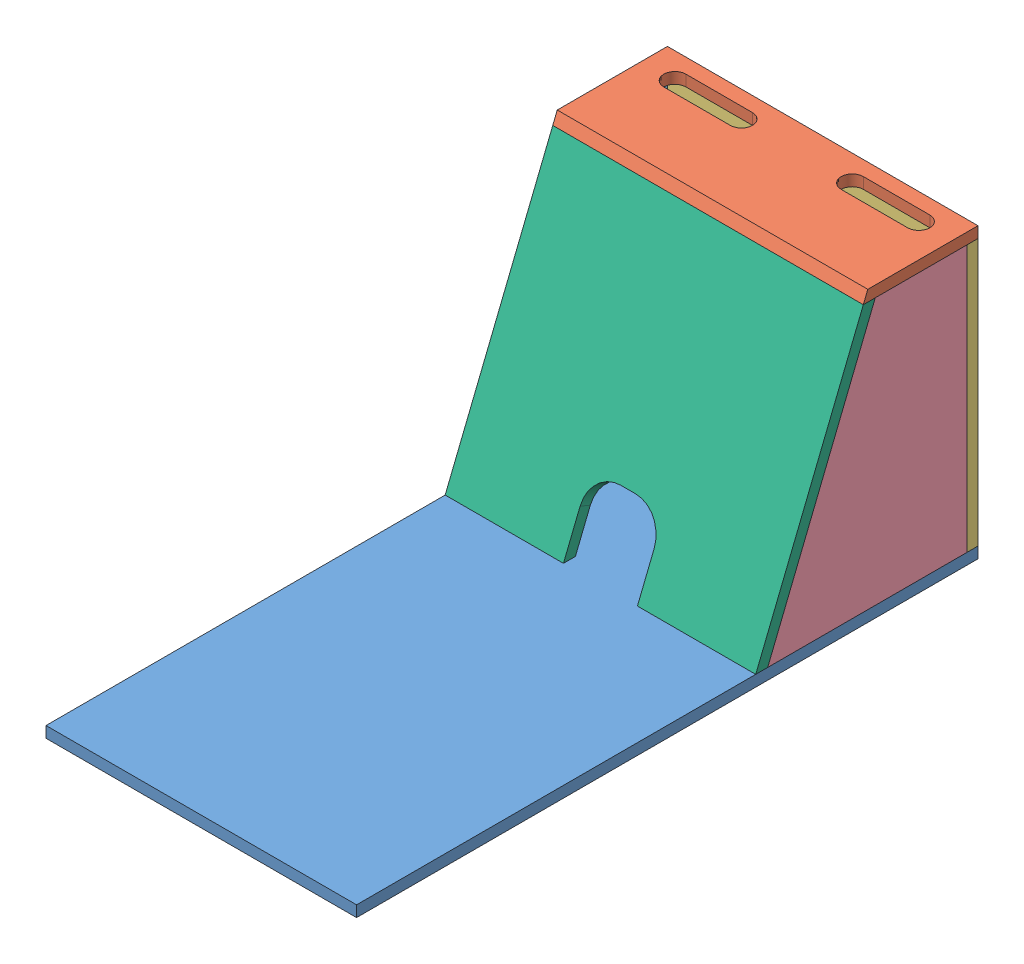
SolidWorks assembly Center Tub, configuration Default. Lengths in mm.
Overall size (533.15 495.3 1066.8).
6 component instances, 6 part files, 17 mates.
Components (placement in the parent):
- Center Tub Floor-1: Center Tub Floor [Default] at (0 2664.46 0) x (-1 0 0) z (0 -1 0) size (533.15 1066.8 19.05)
- Center Tub Keystone-1: Center Tub Keystone [Default] at origin size (533.15 19.05 196.86)
- Center Tub Aft Bulkhead-1: Center Tub Aft Bulkhead [Default] at (0 0 -7002.78) x (-1 0 0) z (0 0 -1) size (533.15 457.2 19.05)
- Center Tub Left Wall-1: Center Tub Left Wall [Default] at (266.573 0 0) x (0 1 0) z (-1 0 0) size (457.2 341.99 19.05)
- Center Tub Right Wall-2: Center Tub Right Wall [Default] at (-266.573 0 0) x (0 1 0) z (-1 0 0) size (457.2 341.99 19.05)
- Center Tub FWD Bulkhead-1: Center Tub FWD Bulkhead [Default] at (-266.573 -1930.2936 -4777.6442) x (0 -0.927184 0.374607) z (0 0.374607 0.927184) size (500.8 533.15 19.05)
Mates (geometry in assembly coordinates):
- InPlace1: in place: plane of ? through (266.7 3017.195 -6812.7359) normal (-1 0 0); plane of ? through (266.7 0 0) normal (-1 0 0); moOrthogonalPlaneRef_w of ? through (266.7 3017.195 -6812.7359) normal (-1 0 0); plane of ? through (266.7 0 0) normal (0 1 0); plane of ? through (266.7 3017.195 -6812.7359) normal (-1 0 0); plane of ? through (266.7 0 0) normal (0 0 1); plane of ? through (266.7 0 0) normal (-1 0 0); unknown of ?
- Coincident1: coincident aligned: plane of ?; plane of assembly
- Coincident2: coincident aligned: plane of Part5^Center Tub-1 through (266.7 0 0) normal (0 0 -1); moOrthogonalPlaneRef_w of Left Console-1/Left Console Structure-1/Inboard Left Console Wall-1 through (266.7 0 0) normal (0 0 -1)
- Coincident3: coincident anti-aligned: plane of Part5^Center Tub-1 through (266.7 0 0) normal (0 1 0); moOrthogonalPlaneRef_w of Left Console-1/Left Console Structure-1/Inboard Left Console Wall-1 through (266.7 0 0) normal (0 -1 0)
- Coincident1: coincident anti-aligned: plane of Center Tub Floor-1 through (0 2683.51 0) normal (0 1 0); plane of Center Tub Left Wall-1 through (247.523 2683.51 -6983.73) normal (0 -1 0)
- Coincident2: coincident aligned: plane of Center Tub Aft Bulkhead-1 through (266.573 2683.51 -6983.73) normal (1 0 0); plane of Center Tub Left Wall-1 through (266.573 0 0) normal (1 0 0)
- Coincident3: coincident anti-aligned: plane of Center Tub Aft Bulkhead-1 through (0 0 -6983.73) normal (0 0 1); plane of Center Tub Left Wall-1 through (247.523 3140.71 -6983.73) normal (0 0 -1)
- InPlace2: in place: plane of ? through (-247.65 2683.51 -6641.7419) normal (0 0.374607 0.927184); plane of ? through (0 -1930.2936 -4777.6442) normal (0 0.374607 0.927184); plane of ? through (-247.65 2683.51 -6641.7419) normal (0 0.374607 0.927184); plane of ? through (0 -1930.2936 -4777.6442) normal (0 0.927184 -0.374607); plane of ? through (-247.65 2683.51 -6641.7419) normal (0 0.374607 0.927184); plane of ? through (0 -1930.2936 -4777.6442) normal (1 0 0); plane of Center Tub Right Wall-2 through (-247.523 2683.51 -6641.7419) normal (0 0.374607 0.927184); unknown of Center Tub FWD Bulkhead-1
- Coincident4: coincident aligned: plane of Center Tub Right Wall-2; plane of Center Tub FWD Bulkhead-1
- Coincident5: coincident aligned: moOrthogonalPlaneRef_w of Center Tub Right Wall-2 through (-266.573 -1930.2936 -4777.6442) normal (1 0 0); plane of Center Tub FWD Bulkhead-1 through (-266.573 -1930.2936 -4777.6442) normal (1 0 0)
- Coincident6: coincident anti-aligned: moOrthogonalPlaneRef_w of Center Tub Right Wall-2 through (-266.573 -1930.2936 -4777.6442) normal (0 0.927184 -0.374607); plane of Center Tub FWD Bulkhead-1 through (-266.573 -1930.2936 -4777.6442) normal (0 -0.927184 0.374607)
- Coincident4: coincident anti-aligned: plane of Center Tub Floor-1 through (0 2683.51 0) normal (0 1 0); plane of Center Tub Aft Bulkhead-1 through (266.573 2683.51 -6983.73) normal (0 -1 0)
- Coincident5: coincident aligned: plane of Center Tub Floor-1 through (-266.573 2683.51 -7002.78) normal (0 0 -1); plane of Center Tub Aft Bulkhead-1 through (0 0 -7002.78) normal (0 0 -1)
- Coincident6: coincident anti-aligned: plane of Center Tub Aft Bulkhead-1 through (0 0 -7002.78) normal (-1 0 0)
- Coincident7: coincident aligned: plane of Center Tub Keystone-1 through (0 0 0) normal (1 0 0)
- Coincident8: coincident aligned: plane of Center Tub Keystone-1 through (266.573 3159.76 -7002.78) normal (0 0 -1); plane of Center Tub Aft Bulkhead-1 through (0 0 -7002.78) normal (0 0 -1)
- Coincident9: coincident anti-aligned: plane of Center Tub Keystone-1 through (0 3140.71 0) normal (0 -1 0); plane of Center Tub Aft Bulkhead-1 through (266.573 3140.71 -6983.73) normal (0 1 0)
